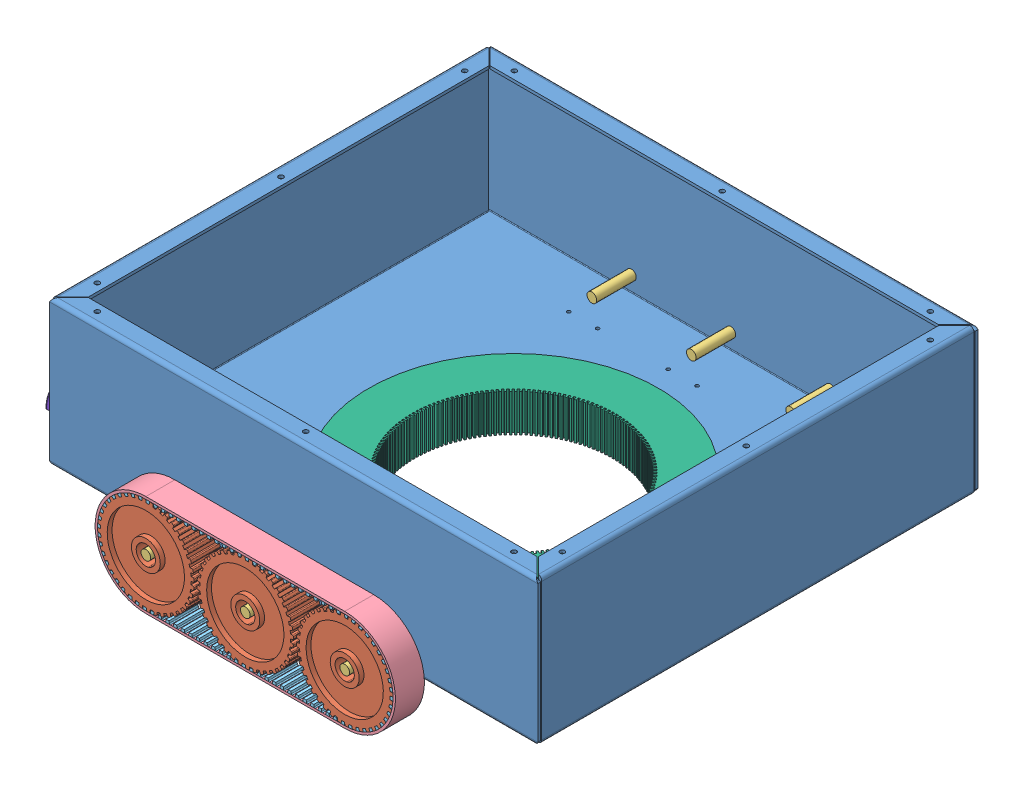
SolidWorks assembly Assem3, configuration Default. Lengths in mm.
Overall size (587.51 201.82 562).
207 component instances, 10 part files, 11 mates.
Components (placement in the parent):
- Base-1: Base [Default] at (139.3424 210.7884 402.3441) size (506.34 150.02 456.02)
- Assem1-1: Assem1 [Default] at (242.3424 61.8445 680.3441) x (0 0 1) z (-1 0 0) size (100 141.1 347.1)
  - geared pully-1: geared pully [Default] at (-15 164.6804 0) x (1 0 0) z (0 0.731888 0.681425) size (30 99.84 99.84)
  - shaft-1: shaft [Default] at (0 164.6804 0) x (0 0 1) z (-1 0 0) size (10 10 100)
  - geared pully-4: geared pully [Default] at (-15 164.6804 103) x (1 0 0) z (0 0.731888 0.681425) size (30 99.84 99.84)
  - geared pully-5: geared pully [Default] at (-15 164.6804 206) x (1 0 0) z (0 0.731888 0.681425) size (30 99.84 99.84)
  - shaft-4: shaft [Default] at (0 164.6804 103) x (0 0 1) z (-1 0 0) size (10 10 100)
  - shaft-5: shaft [Default] at (0 164.6804 206) x (0 0 1) z (-1 0 0) size (10 10 100)
  - Belt1-1^Assem1-1: Belt1-1^Assem1 [Default] at (-2.5 33.9244 206) x (0 0 1) z (-1 0 0) size (311 105 30) (virtual)
  - Part2^Assem1-2: Part2^Assem1 [Default] at (-30 164.6804 0) x (0 0.731888 0.681425) z (-1 0 0) size (3.57 5.71 30) (virtual)
  - Part2^Assem1-121: Part2^Assem1 [Default] at (-30 164.68 0.0008) x (0 0.8299 0.557912) z (-1 0 0) size (3.57 5.71 30) (virtual)
  - Part2^Assem1-122: Part2^Assem1 [Default] at (-30 164.6802 0.0008) x (0 0.907286 0.420515) z (-1 0 0) size (3.57 5.71 30) (virtual)
  - Part2^Assem1-123: Part2^Assem1 [Default] at (-30 164.6803 0.0009) x (0 0.962117 0.272637) z (-1 0 0) size (3.57 5.71 30) (virtual)
  - Part2^Assem1-124: Part2^Assem1 [Default] at (-30 164.6804 2.1565) x (0 0.987006 0.160684) z (-1 0 0) size (3.57 5.71 30) (virtual)
  - Part2^Assem1-125: Part2^Assem1 [Default] at (-30 164.6804 10.0498) x (0 0.987006 0.160684) z (-1 0 0) size (3.57 5.71 30) (virtual)
  - Part2^Assem1-126: Part2^Assem1 [Default] at (-30 164.6804 17.9419) x (0 0.987006 0.160684) z (-1 0 0) size (3.57 5.71 30) (virtual)
  - Part2^Assem1-127: Part2^Assem1 [Default] at (-30 164.6804 25.834) x (0 0.987006 0.160684) z (-1 0 0) size (3.57 5.71 30) (virtual)
  - Part2^Assem1-128: Part2^Assem1 [Default] at (-30 164.6804 33.7272) x (0 0.987006 0.160684) z (-1 0 0) size (3.57 5.71 30) (virtual)
  - Part2^Assem1-129: Part2^Assem1 [Default] at (-30 164.6804 41.6205) x (0 0.987006 0.160684) z (-1 0 0) size (3.57 5.71 30) (virtual)
  - Part2^Assem1-130: Part2^Assem1 [Default] at (-30 164.6804 49.5138) x (0 0.987006 0.160684) z (-1 0 0) size (3.57 5.71 30) (virtual)
  - Part2^Assem1-131: Part2^Assem1 [Default] at (-30 164.6804 57.407) x (0 0.987006 0.160684) z (-1 0 0) size (3.57 5.71 30) (virtual)
  - Part2^Assem1-132: Part2^Assem1 [Default] at (-30 164.6804 65.3003) x (0 0.987006 0.160684) z (-1 0 0) size (3.57 5.71 30) (virtual)
  - Part2^Assem1-133: Part2^Assem1 [Default] at (-30 164.6804 73.1936) x (0 0.987006 0.160684) z (-1 0 0) size (3.57 5.71 30) (virtual)
  - Part2^Assem1-134: Part2^Assem1 [Default] at (-30 164.6804 81.0868) x (0 0.987006 0.160684) z (-1 0 0) size (3.57 5.71 30) (virtual)
  - Part2^Assem1-135: Part2^Assem1 [Default] at (-30 164.6804 88.9801) x (0 0.987006 0.160684) z (-1 0 0) size (3.57 5.71 30) (virtual)
  - Part2^Assem1-136: Part2^Assem1 [Default] at (-30 164.6804 96.8722) x (0 0.987006 0.160684) z (-1 0 0) size (3.57 5.71 30) (virtual)
  - Part2^Assem1-137: Part2^Assem1 [Default] at (-30 164.6804 104.7655) x (0 0.987006 0.160684) z (-1 0 0) size (3.57 5.71 30) (virtual)
  - Part2^Assem1-138: Part2^Assem1 [Default] at (-30 164.6804 112.6575) x (0 0.987006 0.160684) z (-1 0 0) size (3.57 5.71 30) (virtual)
  - Part2^Assem1-139: Part2^Assem1 [Default] at (-30 164.6804 120.5508) x (0 0.987006 0.160684) z (-1 0 0) size (3.57 5.71 30) (virtual)
  - Part2^Assem1-140: Part2^Assem1 [Default] at (-30 164.6804 128.4441) x (0 0.987006 0.160684) z (-1 0 0) size (3.57 5.71 30) (virtual)
  - Part2^Assem1-141: Part2^Assem1 [Default] at (-30 164.6804 136.3373) x (0 0.987006 0.160684) z (-1 0 0) size (3.57 5.71 30) (virtual)
  - Part2^Assem1-142: Part2^Assem1 [Default] at (-30 164.6804 144.2306) x (0 0.987006 0.160684) z (-1 0 0) size (3.57 5.71 30) (virtual)
  - Part2^Assem1-143: Part2^Assem1 [Default] at (-30 164.6804 152.1239) x (0 0.987006 0.160684) z (-1 0 0) size (3.57 5.71 30) (virtual)
  - Part2^Assem1-144: Part2^Assem1 [Default] at (-30 164.6804 160.0171) x (0 0.987006 0.160684) z (-1 0 0) size (3.57 5.71 30) (virtual)
  - Part2^Assem1-145: Part2^Assem1 [Default] at (-30 164.6804 167.9104) x (0 0.987006 0.160684) z (-1 0 0) size (3.57 5.71 30) (virtual)
  - Part2^Assem1-146: Part2^Assem1 [Default] at (-30 164.6804 175.8025) x (0 0.987006 0.160684) z (-1 0 0) size (3.57 5.71 30) (virtual)
  - Part2^Assem1-147: Part2^Assem1 [Default] at (-30 164.6804 183.6958) x (0 0.987006 0.160684) z (-1 0 0) size (3.57 5.71 30) (virtual)
  - Part2^Assem1-148: Part2^Assem1 [Default] at (-30 164.6804 191.5879) x (0 0.987006 0.160684) z (-1 0 0) size (3.57 5.71 30) (virtual)
  - Part2^Assem1-149: Part2^Assem1 [Default] at (-30 164.6804 199.4818) x (0 0.987006 0.160684) z (-1 0 0) size (3.57 5.71 30) (virtual)
  - Part2^Assem1-150: Part2^Assem1 [Default] at (-30 164.6804 206.0056) x (0 0.991038 0.13358) z (-1 0 0) size (3.57 5.71 30) (virtual)
  - Part2^Assem1-151: Part2^Assem1 [Default] at (-30 164.6806 206.0009) x (0 0.999713 -0.023955) z (-1 0 0) size (3.57 5.71 30) (virtual)
  - Part2^Assem1-152: Part2^Assem1 [Default] at (-30 164.6807 206.0008) x (0 0.983517 -0.180816) z (-1 0 0) size (3.57 5.71 30) (virtual)
  - Part2^Assem1-153: Part2^Assem1 [Default] at (-30 164.6808 206.0008) x (0 0.942865 -0.333174) z (-1 0 0) size (3.57 5.71 30) (virtual)
  - Part2^Assem1-154: Part2^Assem1 [Default] at (-30 164.681 206.0007) x (0 0.878753 -0.477278) z (-1 0 0) size (3.57 5.71 30) (virtual)
  - Part2^Assem1-155: Part2^Assem1 [Default] at (-30 164.6811 206.0006) x (0 0.792814 -0.609464) z (-1 0 0) size (3.57 5.71 30) (virtual)
  - Part2^Assem1-156: Part2^Assem1 [Default] at (-30 164.6811 206.0005) x (0 0.687147 -0.726518) z (-1 0 0) size (3.57 5.71 30) (virtual)
  - Part2^Assem1-157: Part2^Assem1 [Default] at (-30 164.6812 206.0004) x (0 0.564382 -0.825513) z (-1 0 0) size (3.57 5.71 30) (virtual)
  - Part2^Assem1-158: Part2^Assem1 [Default] at (-30 164.6813 206.0002) x (0 0.427566 -0.903984) z (-1 0 0) size (3.57 5.71 30) (virtual)
  - Part2^Assem1-159: Part2^Assem1 [Default] at (-30 164.6813 206.0001) x (0 0.280151 -0.959956) z (-1 0 0) size (3.57 5.71 30) (virtual)
  - Part2^Assem1-160: Part2^Assem1 [Default] at (-30 164.6813 206) x (0 0.125769 -0.99206) z (-1 0 0) size (3.57 5.71 30) (virtual)
  - Part2^Assem1-161: Part2^Assem1 [Default] at (-30 164.6813 205.9998) x (0 -0.031765 -0.999495) z (-1 0 0) size (3.57 5.71 30) (virtual)
  - Part2^Assem1-162: Part2^Assem1 [Default] at (-30 164.6812 205.9997) x (0 -0.18849 -0.982075) z (-1 0 0) size (3.57 5.71 30) (virtual)
  - Part2^Assem1-163: Part2^Assem1 [Default] at (-30 164.6812 205.9996) x (0 -0.340527 -0.940235) z (-1 0 0) size (3.57 5.71 30) (virtual)
  - Part2^Assem1-164: Part2^Assem1 [Default] at (-30 164.6811 205.9995) x (0 -0.484101 -0.875012) z (-1 0 0) size (3.57 5.71 30) (virtual)
  - Part2^Assem1-165: Part2^Assem1 [Default] at (-30 164.681 205.9994) x (0 -0.615638 -0.788029) z (-1 0 0) size (3.57 5.71 30) (virtual)
  - Part2^Assem1-166: Part2^Assem1 [Default] at (-30 164.6809 205.9993) x (0 -0.731875 -0.681439) z (-1 0 0) size (3.57 5.71 30) (virtual)
  - Part2^Assem1-167: Part2^Assem1 [Default] at (-30 164.6808 205.9992) x (0 -0.8299 -0.557912) z (-1 0 0) size (3.57 5.71 30) (virtual)
  - Part2^Assem1-168: Part2^Assem1 [Default] at (-30 164.6806 205.9992) x (0 -0.907286 -0.420515) z (-1 0 0) size (3.57 5.71 30) (virtual)
  - Part2^Assem1-169: Part2^Assem1 [Default] at (-30 164.6805 205.9991) x (0 -0.962117 -0.272637) z (-1 0 0) size (3.57 5.71 30) (virtual)
  - Part2^Assem1-170: Part2^Assem1 [Default] at (-30 164.6804 203.845) x (0 -0.987006 -0.160684) z (-1 0 0) size (3.57 5.71 30) (virtual)
  - Part2^Assem1-171: Part2^Assem1 [Default] at (-30 164.6804 195.9502) x (0 -0.987006 -0.160684) z (-1 0 0) size (3.57 5.71 30) (virtual)
  - Part2^Assem1-172: Part2^Assem1 [Default] at (-30 164.6804 188.0581) x (0 -0.987006 -0.160684) z (-1 0 0) size (3.57 5.71 30) (virtual)
  - Part2^Assem1-173: Part2^Assem1 [Default] at (-30 164.6804 180.166) x (0 -0.987006 -0.160684) z (-1 0 0) size (3.57 5.71 30) (virtual)
  - Part2^Assem1-174: Part2^Assem1 [Default] at (-30 164.6804 172.2728) x (0 -0.987006 -0.160684) z (-1 0 0) size (3.57 5.71 30) (virtual)
  - Part2^Assem1-175: Part2^Assem1 [Default] at (-30 164.6804 164.3795) x (0 -0.987006 -0.160684) z (-1 0 0) size (3.57 5.71 30) (virtual)
  - Part2^Assem1-176: Part2^Assem1 [Default] at (-30 164.6804 156.4862) x (0 -0.987006 -0.160684) z (-1 0 0) size (3.57 5.71 30) (virtual)
  - Part2^Assem1-177: Part2^Assem1 [Default] at (-30 164.6804 148.593) x (0 -0.987006 -0.160684) z (-1 0 0) size (3.57 5.71 30) (virtual)
  - Part2^Assem1-178: Part2^Assem1 [Default] at (-30 164.6804 140.6997) x (0 -0.987006 -0.160684) z (-1 0 0) size (3.57 5.71 30) (virtual)
  - Part2^Assem1-179: Part2^Assem1 [Default] at (-30 164.6804 132.8064) x (0 -0.987006 -0.160684) z (-1 0 0) size (3.57 5.71 30) (virtual)
  - Part2^Assem1-180: Part2^Assem1 [Default] at (-30 164.6804 124.9132) x (0 -0.987006 -0.160684) z (-1 0 0) size (3.57 5.71 30) (virtual)
  - Part2^Assem1-181: Part2^Assem1 [Default] at (-30 164.6804 117.0199) x (0 -0.987006 -0.160684) z (-1 0 0) size (3.57 5.71 30) (virtual)
  - Part2^Assem1-182: Part2^Assem1 [Default] at (-30 164.6804 109.1278) x (0 -0.987006 -0.160684) z (-1 0 0) size (3.57 5.71 30) (virtual)
  - Part2^Assem1-183: Part2^Assem1 [Default] at (-30 164.6804 101.2345) x (0 -0.987006 -0.160684) z (-1 0 0) size (3.57 5.71 30) (virtual)
  - Part2^Assem1-184: Part2^Assem1 [Default] at (-30 164.6804 93.3425) x (0 -0.987006 -0.160684) z (-1 0 0) size (3.57 5.71 30) (virtual)
  - Part2^Assem1-185: Part2^Assem1 [Default] at (-30 164.6804 85.4492) x (0 -0.987006 -0.160684) z (-1 0 0) size (3.57 5.71 30) (virtual)
  - Part2^Assem1-186: Part2^Assem1 [Default] at (-30 164.6804 77.5559) x (0 -0.987006 -0.160684) z (-1 0 0) size (3.57 5.71 30) (virtual)
  - Part2^Assem1-187: Part2^Assem1 [Default] at (-30 164.6804 69.6627) x (0 -0.987006 -0.160684) z (-1 0 0) size (3.57 5.71 30) (virtual)
  - Part2^Assem1-188: Part2^Assem1 [Default] at (-30 164.6804 61.7694) x (0 -0.987006 -0.160684) z (-1 0 0) size (3.57 5.71 30) (virtual)
  - Part2^Assem1-189: Part2^Assem1 [Default] at (-30 164.6804 53.8761) x (0 -0.987006 -0.160684) z (-1 0 0) size (3.57 5.71 30) (virtual)
  - Part2^Assem1-190: Part2^Assem1 [Default] at (-30 164.6804 45.9829) x (0 -0.987006 -0.160684) z (-1 0 0) size (3.57 5.71 30) (virtual)
  - Part2^Assem1-191: Part2^Assem1 [Default] at (-30 164.6804 38.0896) x (0 -0.987006 -0.160684) z (-1 0 0) size (3.57 5.71 30) (virtual)
  - Part2^Assem1-192: Part2^Assem1 [Default] at (-30 164.6804 30.1975) x (0 -0.987006 -0.160684) z (-1 0 0) size (3.57 5.71 30) (virtual)
  - Part2^Assem1-193: Part2^Assem1 [Default] at (-30 164.6804 22.3042) x (0 -0.987006 -0.160684) z (-1 0 0) size (3.57 5.71 30) (virtual)
  - Part2^Assem1-194: Part2^Assem1 [Default] at (-30 164.6804 14.4121) x (0 -0.987006 -0.160684) z (-1 0 0) size (3.57 5.71 30) (virtual)
  - Part2^Assem1-195: Part2^Assem1 [Default] at (-30 164.6804 6.5184) x (0 -0.987006 -0.160684) z (-1 0 0) size (3.57 5.71 30) (virtual)
  - Part2^Assem1-196: Part2^Assem1 [Default] at (-30 164.6804 -0.0065) x (0 -0.991032 -0.133625) z (-1 0 0) size (3.57 5.71 30) (virtual)
  - Part2^Assem1-197: Part2^Assem1 [Default] at (-30 164.6802 -0.0009) x (0 -0.999713 0.023955) z (-1 0 0) size (3.57 5.71 30) (virtual)
  - Part2^Assem1-198: Part2^Assem1 [Default] at (-30 164.6801 -0.0008) x (0 -0.983517 0.180816) z (-1 0 0) size (3.57 5.71 30) (virtual)
  - Part2^Assem1-199: Part2^Assem1 [Default] at (-30 164.68 -0.0008) x (0 -0.942865 0.333174) z (-1 0 0) size (3.57 5.71 30) (virtual)
  - Part2^Assem1-200: Part2^Assem1 [Default] at (-30 164.6799 -0.0007) x (0 -0.878753 0.477278) z (-1 0 0) size (3.57 5.71 30) (virtual)
  - Part2^Assem1-201: Part2^Assem1 [Default] at (-30 164.6798 -0.0006) x (0 -0.792814 0.609464) z (-1 0 0) size (3.57 5.71 30) (virtual)
  - Part2^Assem1-202: Part2^Assem1 [Default] at (-30 164.6797 -0.0005) x (0 -0.687147 0.726518) z (-1 0 0) size (3.57 5.71 30) (virtual)
  - Part2^Assem1-203: Part2^Assem1 [Default] at (-30 164.6796 -0.0004) x (0 -0.564382 0.825513) z (-1 0 0) size (3.57 5.71 30) (virtual)
  - Part2^Assem1-204: Part2^Assem1 [Default] at (-30 164.6796 -0.0002) x (0 -0.427566 0.903984) z (-1 0 0) size (3.57 5.71 30) (virtual)
  - Part2^Assem1-205: Part2^Assem1 [Default] at (-30 164.6795 -0.0001) x (0 -0.280151 0.959956) z (-1 0 0) size (3.57 5.71 30) (virtual)
  - Part2^Assem1-206: Part2^Assem1 [Default] at (-30 164.6795 0) x (0 -0.125769 0.99206) z (-1 0 0) size (3.57 5.71 30) (virtual)
  - Part2^Assem1-207: Part2^Assem1 [Default] at (-30 164.6795 0.0002) x (0 0.031765 0.999495) z (-1 0 0) size (3.57 5.71 30) (virtual)
  - Part2^Assem1-208: Part2^Assem1 [Default] at (-30 164.6796 0.0003) x (0 0.18849 0.982075) z (-1 0 0) size (3.57 5.71 30) (virtual)
  - Part2^Assem1-209: Part2^Assem1 [Default] at (-30 164.6796 0.0004) x (0 0.340527 0.940235) z (-1 0 0) size (3.57 5.71 30) (virtual)
  - Part2^Assem1-210: Part2^Assem1 [Default] at (-30 164.6797 0.0005) x (0 0.484101 0.875012) z (-1 0 0) size (3.57 5.71 30) (virtual)
  - Part2^Assem1-211: Part2^Assem1 [Default] at (-30 164.6798 0.0006) x (0 0.615638 0.788029) z (-1 0 0) size (3.57 5.71 30) (virtual)
- Assem1-2: Assem1 [Default] at (36.3424 61.8445 118.3441) x (0 0 -1) z (1 0 0) size (100 141.1 347.1)
  - geared pully-1: geared pully [Default] at (-15 164.6804 0) x (1 0 0) z (0 0.731888 0.681425) size (30 99.84 99.84)
  - shaft-1: shaft [Default] at (0 164.6804 0) x (0 0 1) z (-1 0 0) size (10 10 100)
  - geared pully-4: geared pully [Default] at (-15 164.6804 103) x (1 0 0) z (0 0.731888 0.681425) size (30 99.84 99.84)
  - geared pully-5: geared pully [Default] at (-15 164.6804 206) x (1 0 0) z (0 0.731888 0.681425) size (30 99.84 99.84)
  - shaft-4: shaft [Default] at (0 164.6804 103) x (0 0 1) z (-1 0 0) size (10 10 100)
  - shaft-5: shaft [Default] at (0 164.6804 206) x (0 0 1) z (-1 0 0) size (10 10 100)
  - Belt1-1^Assem1-1: Belt1-1^Assem1 [Default] at (-2.5 33.9244 206) x (0 0 1) z (-1 0 0) size (311 105 30) (virtual)
  - Part2^Assem1-2: Part2^Assem1 [Default] at (-30 164.6804 0) x (0 0.731888 0.681425) z (-1 0 0) size (3.57 5.71 30) (virtual)
  - Part2^Assem1-121: Part2^Assem1 [Default] at (-30 164.68 0.0008) x (0 0.8299 0.557912) z (-1 0 0) size (3.57 5.71 30) (virtual)
  - Part2^Assem1-122: Part2^Assem1 [Default] at (-30 164.6802 0.0008) x (0 0.907286 0.420515) z (-1 0 0) size (3.57 5.71 30) (virtual)
  - Part2^Assem1-123: Part2^Assem1 [Default] at (-30 164.6803 0.0009) x (0 0.962117 0.272637) z (-1 0 0) size (3.57 5.71 30) (virtual)
  - Part2^Assem1-124: Part2^Assem1 [Default] at (-30 164.6804 2.1565) x (0 0.987006 0.160684) z (-1 0 0) size (3.57 5.71 30) (virtual)
  - Part2^Assem1-125: Part2^Assem1 [Default] at (-30 164.6804 10.0498) x (0 0.987006 0.160684) z (-1 0 0) size (3.57 5.71 30) (virtual)
  - Part2^Assem1-126: Part2^Assem1 [Default] at (-30 164.6804 17.9419) x (0 0.987006 0.160684) z (-1 0 0) size (3.57 5.71 30) (virtual)
  - Part2^Assem1-127: Part2^Assem1 [Default] at (-30 164.6804 25.834) x (0 0.987006 0.160684) z (-1 0 0) size (3.57 5.71 30) (virtual)
  - Part2^Assem1-128: Part2^Assem1 [Default] at (-30 164.6804 33.7272) x (0 0.987006 0.160684) z (-1 0 0) size (3.57 5.71 30) (virtual)
  - Part2^Assem1-129: Part2^Assem1 [Default] at (-30 164.6804 41.6205) x (0 0.987006 0.160684) z (-1 0 0) size (3.57 5.71 30) (virtual)
  - Part2^Assem1-130: Part2^Assem1 [Default] at (-30 164.6804 49.5138) x (0 0.987006 0.160684) z (-1 0 0) size (3.57 5.71 30) (virtual)
  - Part2^Assem1-131: Part2^Assem1 [Default] at (-30 164.6804 57.407) x (0 0.987006 0.160684) z (-1 0 0) size (3.57 5.71 30) (virtual)
  - Part2^Assem1-132: Part2^Assem1 [Default] at (-30 164.6804 65.3003) x (0 0.987006 0.160684) z (-1 0 0) size (3.57 5.71 30) (virtual)
  - Part2^Assem1-133: Part2^Assem1 [Default] at (-30 164.6804 73.1936) x (0 0.987006 0.160684) z (-1 0 0) size (3.57 5.71 30) (virtual)
  - Part2^Assem1-134: Part2^Assem1 [Default] at (-30 164.6804 81.0868) x (0 0.987006 0.160684) z (-1 0 0) size (3.57 5.71 30) (virtual)
  - Part2^Assem1-135: Part2^Assem1 [Default] at (-30 164.6804 88.9801) x (0 0.987006 0.160684) z (-1 0 0) size (3.57 5.71 30) (virtual)
  - Part2^Assem1-136: Part2^Assem1 [Default] at (-30 164.6804 96.8722) x (0 0.987006 0.160684) z (-1 0 0) size (3.57 5.71 30) (virtual)
  - Part2^Assem1-137: Part2^Assem1 [Default] at (-30 164.6804 104.7655) x (0 0.987006 0.160684) z (-1 0 0) size (3.57 5.71 30) (virtual)
  - Part2^Assem1-138: Part2^Assem1 [Default] at (-30 164.6804 112.6575) x (0 0.987006 0.160684) z (-1 0 0) size (3.57 5.71 30) (virtual)
  - Part2^Assem1-139: Part2^Assem1 [Default] at (-30 164.6804 120.5508) x (0 0.987006 0.160684) z (-1 0 0) size (3.57 5.71 30) (virtual)
  - Part2^Assem1-140: Part2^Assem1 [Default] at (-30 164.6804 128.4441) x (0 0.987006 0.160684) z (-1 0 0) size (3.57 5.71 30) (virtual)
  - Part2^Assem1-141: Part2^Assem1 [Default] at (-30 164.6804 136.3373) x (0 0.987006 0.160684) z (-1 0 0) size (3.57 5.71 30) (virtual)
  - Part2^Assem1-142: Part2^Assem1 [Default] at (-30 164.6804 144.2306) x (0 0.987006 0.160684) z (-1 0 0) size (3.57 5.71 30) (virtual)
  - Part2^Assem1-143: Part2^Assem1 [Default] at (-30 164.6804 152.1239) x (0 0.987006 0.160684) z (-1 0 0) size (3.57 5.71 30) (virtual)
  - Part2^Assem1-144: Part2^Assem1 [Default] at (-30 164.6804 160.0171) x (0 0.987006 0.160684) z (-1 0 0) size (3.57 5.71 30) (virtual)
  - Part2^Assem1-145: Part2^Assem1 [Default] at (-30 164.6804 167.9104) x (0 0.987006 0.160684) z (-1 0 0) size (3.57 5.71 30) (virtual)
  - Part2^Assem1-146: Part2^Assem1 [Default] at (-30 164.6804 175.8025) x (0 0.987006 0.160684) z (-1 0 0) size (3.57 5.71 30) (virtual)
  - Part2^Assem1-147: Part2^Assem1 [Default] at (-30 164.6804 183.6958) x (0 0.987006 0.160684) z (-1 0 0) size (3.57 5.71 30) (virtual)
  - Part2^Assem1-148: Part2^Assem1 [Default] at (-30 164.6804 191.5879) x (0 0.987006 0.160684) z (-1 0 0) size (3.57 5.71 30) (virtual)
  - Part2^Assem1-149: Part2^Assem1 [Default] at (-30 164.6804 199.4818) x (0 0.987006 0.160684) z (-1 0 0) size (3.57 5.71 30) (virtual)
  - Part2^Assem1-150: Part2^Assem1 [Default] at (-30 164.6804 206.0056) x (0 0.991038 0.13358) z (-1 0 0) size (3.57 5.71 30) (virtual)
  - Part2^Assem1-151: Part2^Assem1 [Default] at (-30 164.6806 206.0009) x (0 0.999713 -0.023955) z (-1 0 0) size (3.57 5.71 30) (virtual)
  - Part2^Assem1-152: Part2^Assem1 [Default] at (-30 164.6807 206.0008) x (0 0.983517 -0.180816) z (-1 0 0) size (3.57 5.71 30) (virtual)
  - Part2^Assem1-153: Part2^Assem1 [Default] at (-30 164.6808 206.0008) x (0 0.942865 -0.333174) z (-1 0 0) size (3.57 5.71 30) (virtual)
  - Part2^Assem1-154: Part2^Assem1 [Default] at (-30 164.681 206.0007) x (0 0.878753 -0.477278) z (-1 0 0) size (3.57 5.71 30) (virtual)
  - Part2^Assem1-155: Part2^Assem1 [Default] at (-30 164.6811 206.0006) x (0 0.792814 -0.609464) z (-1 0 0) size (3.57 5.71 30) (virtual)
  - Part2^Assem1-156: Part2^Assem1 [Default] at (-30 164.6811 206.0005) x (0 0.687147 -0.726518) z (-1 0 0) size (3.57 5.71 30) (virtual)
  - Part2^Assem1-157: Part2^Assem1 [Default] at (-30 164.6812 206.0004) x (0 0.564382 -0.825513) z (-1 0 0) size (3.57 5.71 30) (virtual)
  - Part2^Assem1-158: Part2^Assem1 [Default] at (-30 164.6813 206.0002) x (0 0.427566 -0.903984) z (-1 0 0) size (3.57 5.71 30) (virtual)
  - Part2^Assem1-159: Part2^Assem1 [Default] at (-30 164.6813 206.0001) x (0 0.280151 -0.959956) z (-1 0 0) size (3.57 5.71 30) (virtual)
  - Part2^Assem1-160: Part2^Assem1 [Default] at (-30 164.6813 206) x (0 0.125769 -0.99206) z (-1 0 0) size (3.57 5.71 30) (virtual)
  - Part2^Assem1-161: Part2^Assem1 [Default] at (-30 164.6813 205.9998) x (0 -0.031765 -0.999495) z (-1 0 0) size (3.57 5.71 30) (virtual)
  - Part2^Assem1-162: Part2^Assem1 [Default] at (-30 164.6812 205.9997) x (0 -0.18849 -0.982075) z (-1 0 0) size (3.57 5.71 30) (virtual)
  - Part2^Assem1-163: Part2^Assem1 [Default] at (-30 164.6812 205.9996) x (0 -0.340527 -0.940235) z (-1 0 0) size (3.57 5.71 30) (virtual)
  - Part2^Assem1-164: Part2^Assem1 [Default] at (-30 164.6811 205.9995) x (0 -0.484101 -0.875012) z (-1 0 0) size (3.57 5.71 30) (virtual)
  - Part2^Assem1-165: Part2^Assem1 [Default] at (-30 164.681 205.9994) x (0 -0.615638 -0.788029) z (-1 0 0) size (3.57 5.71 30) (virtual)
  - Part2^Assem1-166: Part2^Assem1 [Default] at (-30 164.6809 205.9993) x (0 -0.731875 -0.681439) z (-1 0 0) size (3.57 5.71 30) (virtual)
  - Part2^Assem1-167: Part2^Assem1 [Default] at (-30 164.6808 205.9992) x (0 -0.8299 -0.557912) z (-1 0 0) size (3.57 5.71 30) (virtual)
  - Part2^Assem1-168: Part2^Assem1 [Default] at (-30 164.6806 205.9992) x (0 -0.907286 -0.420515) z (-1 0 0) size (3.57 5.71 30) (virtual)
  - Part2^Assem1-169: Part2^Assem1 [Default] at (-30 164.6805 205.9991) x (0 -0.962117 -0.272637) z (-1 0 0) size (3.57 5.71 30) (virtual)
  - Part2^Assem1-170: Part2^Assem1 [Default] at (-30 164.6804 203.845) x (0 -0.987006 -0.160684) z (-1 0 0) size (3.57 5.71 30) (virtual)
  - Part2^Assem1-171: Part2^Assem1 [Default] at (-30 164.6804 195.9502) x (0 -0.987006 -0.160684) z (-1 0 0) size (3.57 5.71 30) (virtual)
  - Part2^Assem1-172: Part2^Assem1 [Default] at (-30 164.6804 188.0581) x (0 -0.987006 -0.160684) z (-1 0 0) size (3.57 5.71 30) (virtual)
  - Part2^Assem1-173: Part2^Assem1 [Default] at (-30 164.6804 180.166) x (0 -0.987006 -0.160684) z (-1 0 0) size (3.57 5.71 30) (virtual)
  - Part2^Assem1-174: Part2^Assem1 [Default] at (-30 164.6804 172.2728) x (0 -0.987006 -0.160684) z (-1 0 0) size (3.57 5.71 30) (virtual)
  - Part2^Assem1-175: Part2^Assem1 [Default] at (-30 164.6804 164.3795) x (0 -0.987006 -0.160684) z (-1 0 0) size (3.57 5.71 30) (virtual)
  - Part2^Assem1-176: Part2^Assem1 [Default] at (-30 164.6804 156.4862) x (0 -0.987006 -0.160684) z (-1 0 0) size (3.57 5.71 30) (virtual)
  - Part2^Assem1-177: Part2^Assem1 [Default] at (-30 164.6804 148.593) x (0 -0.987006 -0.160684) z (-1 0 0) size (3.57 5.71 30) (virtual)
  - Part2^Assem1-178: Part2^Assem1 [Default] at (-30 164.6804 140.6997) x (0 -0.987006 -0.160684) z (-1 0 0) size (3.57 5.71 30) (virtual)
  - Part2^Assem1-179: Part2^Assem1 [Default] at (-30 164.6804 132.8064) x (0 -0.987006 -0.160684) z (-1 0 0) size (3.57 5.71 30) (virtual)
  - Part2^Assem1-180: Part2^Assem1 [Default] at (-30 164.6804 124.9132) x (0 -0.987006 -0.160684) z (-1 0 0) size (3.57 5.71 30) (virtual)
  - Part2^Assem1-181: Part2^Assem1 [Default] at (-30 164.6804 117.0199) x (0 -0.987006 -0.160684) z (-1 0 0) size (3.57 5.71 30) (virtual)
  - Part2^Assem1-182: Part2^Assem1 [Default] at (-30 164.6804 109.1278) x (0 -0.987006 -0.160684) z (-1 0 0) size (3.57 5.71 30) (virtual)
  - Part2^Assem1-183: Part2^Assem1 [Default] at (-30 164.6804 101.2345) x (0 -0.987006 -0.160684) z (-1 0 0) size (3.57 5.71 30) (virtual)
  - Part2^Assem1-184: Part2^Assem1 [Default] at (-30 164.6804 93.3425) x (0 -0.987006 -0.160684) z (-1 0 0) size (3.57 5.71 30) (virtual)
  - Part2^Assem1-185: Part2^Assem1 [Default] at (-30 164.6804 85.4492) x (0 -0.987006 -0.160684) z (-1 0 0) size (3.57 5.71 30) (virtual)
  - Part2^Assem1-186: Part2^Assem1 [Default] at (-30 164.6804 77.5559) x (0 -0.987006 -0.160684) z (-1 0 0) size (3.57 5.71 30) (virtual)
  - Part2^Assem1-187: Part2^Assem1 [Default] at (-30 164.6804 69.6627) x (0 -0.987006 -0.160684) z (-1 0 0) size (3.57 5.71 30) (virtual)
  - Part2^Assem1-188: Part2^Assem1 [Default] at (-30 164.6804 61.7694) x (0 -0.987006 -0.160684) z (-1 0 0) size (3.57 5.71 30) (virtual)
  - Part2^Assem1-189: Part2^Assem1 [Default] at (-30 164.6804 53.8761) x (0 -0.987006 -0.160684) z (-1 0 0) size (3.57 5.71 30) (virtual)
  - Part2^Assem1-190: Part2^Assem1 [Default] at (-30 164.6804 45.9829) x (0 -0.987006 -0.160684) z (-1 0 0) size (3.57 5.71 30) (virtual)
  - Part2^Assem1-191: Part2^Assem1 [Default] at (-30 164.6804 38.0896) x (0 -0.987006 -0.160684) z (-1 0 0) size (3.57 5.71 30) (virtual)
  - Part2^Assem1-192: Part2^Assem1 [Default] at (-30 164.6804 30.1975) x (0 -0.987006 -0.160684) z (-1 0 0) size (3.57 5.71 30) (virtual)
  - Part2^Assem1-193: Part2^Assem1 [Default] at (-30 164.6804 22.3042) x (0 -0.987006 -0.160684) z (-1 0 0) size (3.57 5.71 30) (virtual)
  - Part2^Assem1-194: Part2^Assem1 [Default] at (-30 164.6804 14.4121) x (0 -0.987006 -0.160684) z (-1 0 0) size (3.57 5.71 30) (virtual)
  - Part2^Assem1-195: Part2^Assem1 [Default] at (-30 164.6804 6.5184) x (0 -0.987006 -0.160684) z (-1 0 0) size (3.57 5.71 30) (virtual)
  - Part2^Assem1-196: Part2^Assem1 [Default] at (-30 164.6804 -0.0065) x (0 -0.991032 -0.133625) z (-1 0 0) size (3.57 5.71 30) (virtual)
  - Part2^Assem1-197: Part2^Assem1 [Default] at (-30 164.6802 -0.0009) x (0 -0.999713 0.023955) z (-1 0 0) size (3.57 5.71 30) (virtual)
  - Part2^Assem1-198: Part2^Assem1 [Default] at (-30 164.6801 -0.0008) x (0 -0.983517 0.180816) z (-1 0 0) size (3.57 5.71 30) (virtual)
  - Part2^Assem1-199: Part2^Assem1 [Default] at (-30 164.68 -0.0008) x (0 -0.942865 0.333174) z (-1 0 0) size (3.57 5.71 30) (virtual)
  - Part2^Assem1-200: Part2^Assem1 [Default] at (-30 164.6799 -0.0007) x (0 -0.878753 0.477278) z (-1 0 0) size (3.57 5.71 30) (virtual)
  - Part2^Assem1-201: Part2^Assem1 [Default] at (-30 164.6798 -0.0006) x (0 -0.792814 0.609464) z (-1 0 0) size (3.57 5.71 30) (virtual)
  - Part2^Assem1-202: Part2^Assem1 [Default] at (-30 164.6797 -0.0005) x (0 -0.687147 0.726518) z (-1 0 0) size (3.57 5.71 30) (virtual)
  - Part2^Assem1-203: Part2^Assem1 [Default] at (-30 164.6796 -0.0004) x (0 -0.564382 0.825513) z (-1 0 0) size (3.57 5.71 30) (virtual)
  - Part2^Assem1-204: Part2^Assem1 [Default] at (-30 164.6796 -0.0002) x (0 -0.427566 0.903984) z (-1 0 0) size (3.57 5.71 30) (virtual)
  - Part2^Assem1-205: Part2^Assem1 [Default] at (-30 164.6795 -0.0001) x (0 -0.280151 0.959956) z (-1 0 0) size (3.57 5.71 30) (virtual)
  - Part2^Assem1-206: Part2^Assem1 [Default] at (-30 164.6795 0) x (0 -0.125769 0.99206) z (-1 0 0) size (3.57 5.71 30) (virtual)
  - Part2^Assem1-207: Part2^Assem1 [Default] at (-30 164.6795 0.0002) x (0 0.031765 0.999495) z (-1 0 0) size (3.57 5.71 30) (virtual)
  - Part2^Assem1-208: Part2^Assem1 [Default] at (-30 164.6796 0.0003) x (0 0.18849 0.982075) z (-1 0 0) size (3.57 5.71 30) (virtual)
  - Part2^Assem1-209: Part2^Assem1 [Default] at (-30 164.6796 0.0004) x (0 0.340527 0.940235) z (-1 0 0) size (3.57 5.71 30) (virtual)
  - Part2^Assem1-210: Part2^Assem1 [Default] at (-30 164.6797 0.0005) x (0 0.484101 0.875012) z (-1 0 0) size (3.57 5.71 30) (virtual)
  - Part2^Assem1-211: Part2^Assem1 [Default] at (-30 164.6798 0.0006) x (0 0.615638 0.788029) z (-1 0 0) size (3.57 5.71 30) (virtual)
- skirt sealing-1: skirt sealing [Default] at (139.3424 213.7884 402.3441) x (-0.837169 0 -0.546944) z (-0.546944 0 0.837169) size (300 39 300)
- cleaning part-1: cleaning part [Default] at (-175.8312 52.1239 502.2369) x (1 0 0) z (0 1 0) size (115.57 320 56.98)
  - holder2-1: holder2 [Default] at (565.4382 75.7061 153.1645) size (72.07 200 12.5)
  - Part3-1: Part3 [Default] at (47.6736 218.1083 165.1645) x (-1 0 0) z (0 0 1) size (62 307 39.51)
  - brush 2-2: brush 2 [Default] at (24.6736 252.0044 137.1645) x (1 0 0) z (0 -1 0) size (52.04 51.98 320)
- champer-1: champer [Default] at (139.3424 178.7884 402.3441) size (400 29 400)
Mates (geometry in assembly coordinates):
- Concentric1: concentric aligned: cylinder of Base-1 through (242.3424 226.525 174.3366) axis (0 0 1) radius 5; cylinder of Assem1-1/shaft-1 through (242.3424 226.525 580.3441) axis (0 0 1) radius 5
- Concentric2: concentric aligned: cylinder of Base-1 through (139.3424 226.525 174.3366) axis (0 0 1) radius 5; cylinder of Assem1-1/shaft-4 through (139.3424 226.525 580.3441) axis (0 0 1) radius 5
- Concentric3: concentric aligned: cylinder of Base-1 through (36.3424 226.525 174.3366) axis (0 0 1) radius 5; cylinder of Assem1-1/shaft-5 through (36.3424 226.525 580.3441) axis (0 0 1) radius 5
- Distance1: distance = 20 mm anti-aligned: plane of Assem1-1/geared pully-5 through (47.3207 236.7463 650.3441) normal (0 0 -1); plane of Base-1 through (139.3424 210.7884 630.3441) normal (0 0 1)
- Concentric4: concentric anti-aligned: cylinder of Base-1 through (139.3424 207.7798 402.3441) axis (0 1 0) radius 111.25; cylinder of skirt sealing-1 through (139.3424 111.7226 402.3441) axis (0 -1 0) radius 112.5
- Coincident1: coincident anti-aligned: plane of Base-1 through (139.3424 210.7884 402.3441) normal (0 1 0); plane of skirt sealing-1 through (13.767 210.7884 320.3025) normal (0 -1 0)
- Coincident3: coincident aligned: plane of Base-1 through (139.3424 207.7884 402.3441) normal (0 -1 0); plane of cleaning part-1/holder2-1 through (133.357 207.7884 399.0056) normal (0 -1 0)
- Distance2: distance = 18 mm anti-aligned: plane of cleaning part-1/holder2-1 through (-131.6576 205.2884 426.5308) normal (1 0 0); plane of Base-1 through (-113.6576 210.7884 402.3441) normal (-1 0 0)
- Distance3: distance = 76.6116 mm aligned: plane of cleaning part-1/Part3-1 through (-133.1576 217.2884 553.7325) normal (0 0 1); plane of Base-1 through (139.3424 210.7884 630.3441) normal (0 0 1)
- Coincident7: coincident anti-aligned: plane of Base-1 through (139.3424 207.7884 402.3441) normal (0 -1 0); plane of champer-1 through (139.3424 207.7884 402.3441) normal (0 1 0)
- Concentric5: concentric aligned: cylinder of skirt sealing-1 through (139.3424 111.7226 402.3441) axis (0 -1 0) radius 112.5; cylinder of champer-1 through (139.3424 207.7884 402.3441) axis (0 -1 0) radius 112.5
